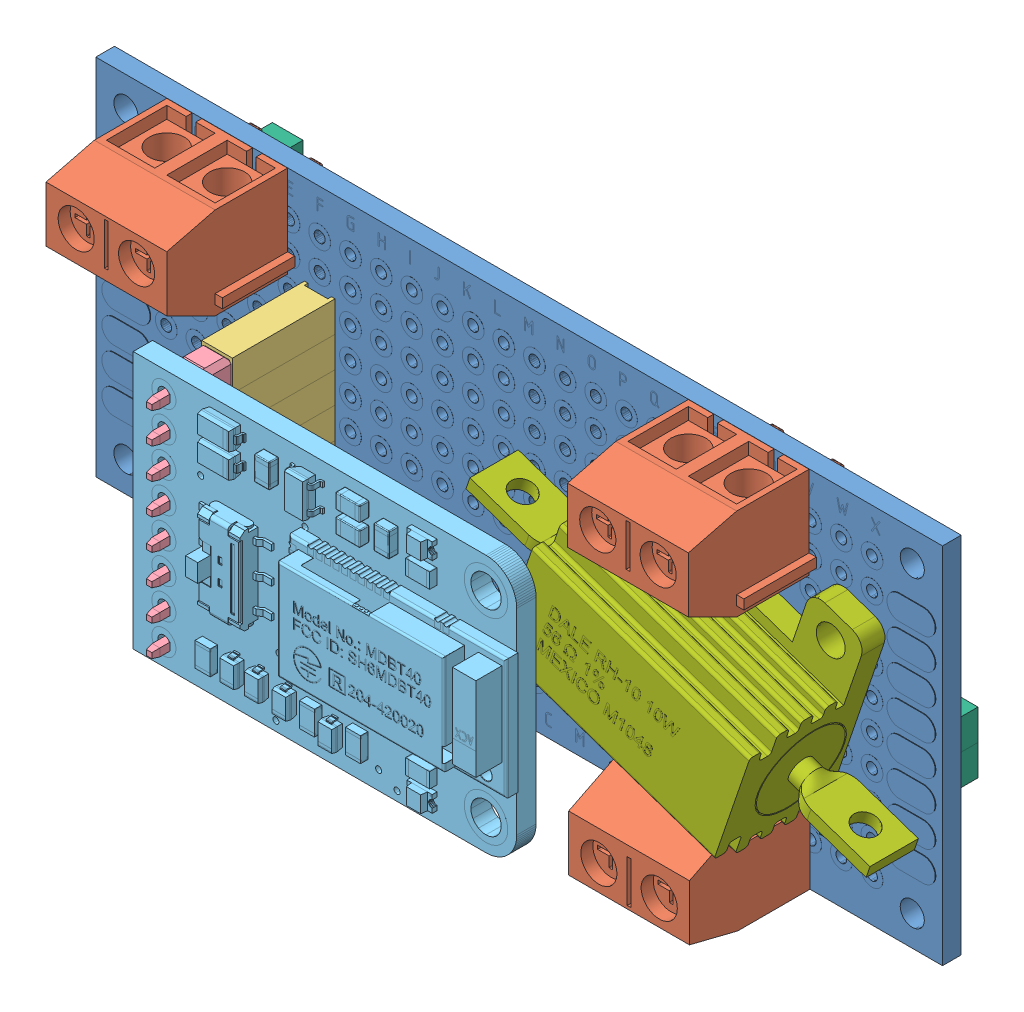
SolidWorks assembly BLEShuntPCB, configuration Default. Lengths in mm.
Overall size (73.24 30.62 25.87).
19 component instances, 7 part files, 42 mates.
Components (placement in the parent):
- 3x7PerfBoard-1: 3x7PerfBoard [Default] at origin size (70.1 30.1 1.65)
- 5mm2PTerminalBlock-1: 5mm2PTerminalBlock [Default] at (-19.17 15.03 1.55) x (-1 0 0) z (0 0 1) size (10.6 7.6 15)
- FemalePinHeader8By1.stp-1: FemalePinHeader8By1.stp [Default] at (-16.51 6.35 1.55) x (0 -1 0) z (0 0 1) size (20.32 2.54 11.7)
  - Female Pin Header 1x.stp-1: Female Pin Header 1x.stp [Default] at origin size (2.54 2.54 11.7)
  - Female Pin Header 1x.stp-2: Female Pin Header 1x.stp [Default] at (2.54 0 0) size (2.54 2.54 11.7)
  - Female Pin Header 1x.stp-3: Female Pin Header 1x.stp [Default] at (5.08 0 0) size (2.54 2.54 11.7)
  - Female Pin Header 1x.stp-4: Female Pin Header 1x.stp [Default] at (7.62 0 0) size (2.54 2.54 11.7)
  - Female Pin Header 1x.stp-5: Female Pin Header 1x.stp [Default] at (10.16 0 0) size (2.54 2.54 11.7)
  - Female Pin Header 1x.stp-6: Female Pin Header 1x.stp [Default] at (12.7 0 0) size (2.54 2.54 11.7)
  - Female Pin Header 1x.stp-7: Female Pin Header 1x.stp [Default] at (15.24 0 0) size (2.54 2.54 11.7)
  - Female Pin Header 1x.stp-8: Female Pin Header 1x.stp [Default] at (17.78 0 0) size (2.54 2.54 11.7)
- 1x8 Male Pin Header.step-1: 1x8 Male Pin Header.step [Default] at (-16.59 6.27 12.59) x (0 -1 0) z (1 0 0) size (20.32 13.54 2.5)
- BLEFriend.stp-1: BLEFriend.stp [Default] at (-19.31 8.128 12.59) x (0 -1 0) z (0 0 1) size (21.35 31.87 4.78)
- 5mm2PTerminalBlock-2: 5mm2PTerminalBlock [Default] at (24.01 15.03 1.55) x (-1 0 0) z (0 0 1) size (10.6 7.6 15)
- 5mm2PTerminalBlock-5: 5mm2PTerminalBlock [Default] at (14.1 -15.03 1.55) size (10.6 7.6 15)
- FemalePinHeader2By1-1: FemalePinHeader2By1 [Default] at (-29.21 -8.89 0) x (0 -1 0) z (0 0 -1) size (5.08 2.54 11.7)
- FemalePinHeader2By1-2: FemalePinHeader2By1 [Default] at (-29.21 6.35 0) x (0 -1 0) z (0 0 -1) size (5.08 2.54 11.7)
- FemalePinHeader2By1-3: FemalePinHeader2By1 [Default] at (26.67 -6.35 0) x (0 -1 0) z (0 0 -1) size (5.08 2.54 11.7)
- ShuntResistor-1: ShuntResistor [Default<As Machined>] at (18.3281 0.2483 1.55) x (0.946299 -0.323291 0) z (-0.323291 -0.946299 0) size (35 9.71 20.4)
Mates (geometry in assembly coordinates):
- Coincident1: coincident aligned: plane of 3x7PerfBoard-1 through (0 0 0) normal (0 0 1)
- Coincident2: coincident aligned: plane of 3x7PerfBoard-1 through (0 0 0) normal (0 1 0)
- Coincident3: coincident aligned: plane of 3x7PerfBoard-1 through (0 0 0) normal (1 0 0)
- Parallel1: parallel aligned: plane of 3x7PerfBoard-1 through (-35.05 15.05 0) normal (0 1 0); plane of 5mm2PTerminalBlock-1 through (-19.17 15.03 1.55) normal (0 1 0)
- Width1: width: cylinder of 5mm2PTerminalBlock-1; plane of 3x7PerfBoard-1 through (-26.27 11.93 -3.45) normal (1 0 0); cylinder of 5mm2PTerminalBlock-1 through (-26.67 11.43 0) axis (0 0 -1) radius 0.45
- Width2: width: plane of 5mm2PTerminalBlock-1 through (-21.27 11.93 -3.45) normal (0 1 0); plane of 3x7PerfBoard-1 through (-21.27 10.93 -3.45) normal (0 -1 0); cylinder of 5mm2PTerminalBlock-1 through (-26.67 11.43 0) axis (0 0 -1) radius 0.45
- Coincident5: coincident anti-aligned: plane of 3x7PerfBoard-1 through (0 0 1.55) normal (0 0 1); plane of 5mm2PTerminalBlock-1 through (-19.17 15.03 1.55) normal (0 0 -1)
- Parallel2: parallel aligned: plane of 3x7PerfBoard-1 through (35.05 -15.05 0) normal (0 -1 0); plane of FemalePinHeader8By1.stp-1/Female Pin Header 1x.stp-8 through (-17.78 -12.7 1.55) normal (0 -1 0)
- Coincident7: coincident anti-aligned: plane of 3x7PerfBoard-1 through (0 0 1.55) normal (0 0 1); plane of FemalePinHeader8By1.stp-1/Female Pin Header 1x.stp-8 through (-16.51 -11.43 1.55) normal (0 0 -1)
- Width3: width: plane of FemalePinHeader8By1.stp-1/Female Pin Header 1x.stp-8 through (-16.31 -12.53 1.55) normal (1 0 0); plane of 3x7PerfBoard-1 through (-16.71 -10.33 1.55) normal (-1 0 0); cylinder of FemalePinHeader8By1.stp-1/Female Pin Header 1x.stp-8 through (-16.51 -11.43 0) axis (0 0 -1) radius 0.45
- Width4: width: plane of FemalePinHeader8By1.stp-1/Female Pin Header 1x.stp-8 through (-16.71 -11.755 -1.65) normal (0 -1 0); plane of 3x7PerfBoard-1 through (-16.71 -11.105 2.35) normal (0 1 0); cylinder of FemalePinHeader8By1.stp-1/Female Pin Header 1x.stp-8 through (-16.51 -11.43 0) axis (0 0 -1) radius 0.45
- Coincident8: coincident anti-aligned: plane of FemalePinHeader8By1.stp-1/Female Pin Header 1x.stp-7 through (-16.51 -8.89 10.05) normal (0 0 1); plane of 1x8 Male Pin Header.step-1 through (-16.59 -3.89 10.05) normal (0 0 -1)
- Coincident9: coincident anti-aligned: plane of FemalePinHeader8By1.stp-1/Female Pin Header 1x.stp-8 through (-16.11 -11.83 10.05) normal (0 1 0); plane of 1x8 Male Pin Header.step-1 through (-16.27 -11.83 2.05) normal (0 -1 0)
- Coincident10: coincident anti-aligned: plane of FemalePinHeader8By1.stp-1/Female Pin Header 1x.stp-8 through (-16.91 -11.83 10.05) normal (1 0 0); plane of 1x8 Male Pin Header.step-1 through (-16.91 -11.19 2.05) normal (-1 0 0)
- Coincident11: coincident anti-aligned: plane of 1x8 Male Pin Header.step-1 through (-16.59 6.27 12.59) normal (0 0 1); plane of BLEFriend.stp-1 through (12.44 8.128 12.59) normal (0 0 -1)
- Tangent1: tangent: plane of 1x8 Male Pin Header.step-1 through (-16.27 -11.19 2.05) normal (1 0 0); curve of BLEFriend.stp-1
- Tangent2: tangent: plane of 1x8 Male Pin Header.step-1 through (-16.27 6.59 2.05) normal (1 0 0); curve of BLEFriend.stp-1
- Symmetric1: symmetric aligned: plane of FemalePinHeader8By1.stp-1/Female Pin Header 1x.stp-4 through (-17.78 -2.54 1.55) normal (0 -1 0); plane of BLEFriend.stp-1 through (9.9 8.128 14.19) normal (0 1 0); plane of BLEFriend.stp-1 through (9.9 -13.208 12.59) normal (0 -1 0)
- Width5: width: plane of 5mm2PTerminalBlock-2 through (16.11 11.93 -3.45) normal (-1 0 0); plane of 3x7PerfBoard-1 through (16.91 11.93 -3.45) normal (1 0 0); cylinder of 5mm2PTerminalBlock-2 through (16.51 11.43 0) axis (0 0 -1) radius 0.45
- Width6: width: plane of 5mm2PTerminalBlock-2 through (21.91 11.93 -3.45) normal (0 1 0); plane of 3x7PerfBoard-1 through (21.91 10.93 -3.45) normal (0 -1 0); cylinder of 5mm2PTerminalBlock-2 through (16.52 11.43 -0.005) axis (0 0 -1) radius 0.45
- Coincident12: coincident anti-aligned: plane of 3x7PerfBoard-1 through (0 0 1.55) normal (0 0 1); plane of 5mm2PTerminalBlock-2 through (24.01 15.03 1.55) normal (0 0 -1)
- Parallel3: parallel aligned: plane of 3x7PerfBoard-1 through (-35.05 15.05 0) normal (0 1 0); plane of 5mm2PTerminalBlock-2 through (24.01 15.03 1.55) normal (0 1 0)
- Parallel6: parallel aligned: plane of 3x7PerfBoard-1 through (35.05 -15.05 0) normal (0 -1 0); plane of 5mm2PTerminalBlock-5 through (14.1 -15.03 1.55) normal (0 -1 0)
- Coincident14: coincident anti-aligned: plane of 3x7PerfBoard-1 through (0 0 1.55) normal (0 0 1); plane of 5mm2PTerminalBlock-5 through (14.1 -15.03 1.55) normal (0 0 -1)
- Width10: width: plane of 5mm2PTerminalBlock-5 through (16.2 -11.93 -3.45) normal (0 -1 0); plane of 3x7PerfBoard-1 through (16.2 -10.93 -3.45) normal (0 1 0); cylinder of 5mm2PTerminalBlock-5 through (29.21 -11.43 0) axis (0 0 -1) radius 0.45
- Width11: width: plane of 5mm2PTerminalBlock-5 through (22 -11.93 -3.45) normal (1 0 0); plane of 3x7PerfBoard-1 through (21.2 -11.93 -3.45) normal (-1 0 0); cylinder of 5mm2PTerminalBlock-5 through (21.6 -11.43 -0.005) axis (0 0 -1) radius 0.45
- Coincident15: coincident anti-aligned: plane of 3x7PerfBoard-1 through (0 0 0) normal (0 0 -1); plane of FemalePinHeader2By1-1 through (-29.21 -8.89 0) normal (0 0 1)
- Width12: width: plane of FemalePinHeader2By1-1 through (-29.01 -10.33 0) normal (1 0 0); plane of FemalePinHeader2By1-1 through (-29.41 -12.53 0) normal (-1 0 0); cylinder of 3x7PerfBoard-1 through (-29.21 -11.43 -0.005) axis (0 0 -1) radius 0.45
- Width13: width: plane of FemalePinHeader2By1-1 through (-29.01 -11.755 3.2) normal (0 -1 0); plane of FemalePinHeader2By1-1 through (-29.01 -11.105 -0.8) normal (0 1 0); cylinder of 3x7PerfBoard-1 through (-29.21 -11.43 -0.005) axis (0 0 -1) radius 0.45
- Parallel7: parallel aligned: plane of 3x7PerfBoard-1 through (35.05 -15.05 0) normal (0 -1 0); plane of FemalePinHeader2By1-1 through (-27.94 -12.7 0) normal (0 -1 0)
- Coincident17: coincident anti-aligned: plane of 3x7PerfBoard-1 through (0 0 0) normal (0 0 -1); plane of FemalePinHeader2By1-2 through (-29.21 6.35 0) normal (0 0 1)
- Parallel8: parallel aligned: plane of 3x7PerfBoard-1 through (35.05 -15.05 0) normal (0 -1 0); plane of FemalePinHeader2By1-2 through (-27.94 2.54 0) normal (0 -1 0)
- Width15: width: plane of FemalePinHeader2By1-2 through (-29.01 4.91 0) normal (1 0 0); plane of FemalePinHeader2By1-2 through (-29.41 2.71 0) normal (-1 0 0); cylinder of 3x7PerfBoard-1 through (-29.21 -11.43 -0.005) axis (0 0 -1) radius 0.45
- Width16: width: plane of FemalePinHeader2By1-2 through (-29.01 3.485 3.2) normal (0 -1 0); plane of FemalePinHeader2By1-2 through (-29.01 4.135 -0.8) normal (0 1 0); cylinder of 3x7PerfBoard-1 through (-29.21 3.81 0) axis (0 0 -1) radius 0.45
- Coincident18: coincident anti-aligned: plane of 3x7PerfBoard-1 through (0 0 0) normal (0 0 -1); plane of FemalePinHeader2By1-3 through (26.67 -6.35 0) normal (0 0 1)
- Parallel9: parallel aligned: plane of 3x7PerfBoard-1 through (35.05 -15.05 0) normal (0 -1 0); plane of FemalePinHeader2By1-3 through (27.94 -10.16 0) normal (0 -1 0)
- Width18: width: plane of FemalePinHeader2By1-3 through (26.87 -9.215 3.2) normal (0 -1 0); plane of FemalePinHeader2By1-3 through (26.87 -8.565 -0.8) normal (0 1 0); cylinder of 3x7PerfBoard-1 through (26.68 -8.89 -0.005) axis (0 0 -1) radius 0.45
- Width19: width: plane of FemalePinHeader2By1-3 through (26.87 -7.79 0) normal (1 0 0); plane of FemalePinHeader2By1-3 through (26.47 -9.99 0) normal (-1 0 0); cylinder of 3x7PerfBoard-1 through (26.67 -11.43 0) axis (0 0 -1) radius 0.45
- Coincident19: coincident anti-aligned: plane of 3x7PerfBoard-1 through (0 0 1.55) normal (0 0 1); plane of ShuntResistor-1 through (26.8209 6.8576 1.55) normal (0 0 -1)
- Coincident20: coincident: line of 5mm2PTerminalBlock-2 through (14.01 7.43 1.55) axis (0 0 1); plane of ShuntResistor-1 through (11.084 8.4296 3.45) normal (0.323291 0.946299 0)
- Coincident21: coincident: line of 5mm2PTerminalBlock-5 through (24.1 -7.43 1.55) axis (0 0 1); plane of ShuntResistor-1 through (12.1347 -3.3422 3.45) normal (-0.323291 -0.946299 0)
- Coincident22: coincident: plane of 3x7PerfBoard-1 through (35.05 15.05 0) normal (1 0 0); line of ShuntResistor-1 through (35.05 -4.9361 7.55) axis (0 0 -1)
